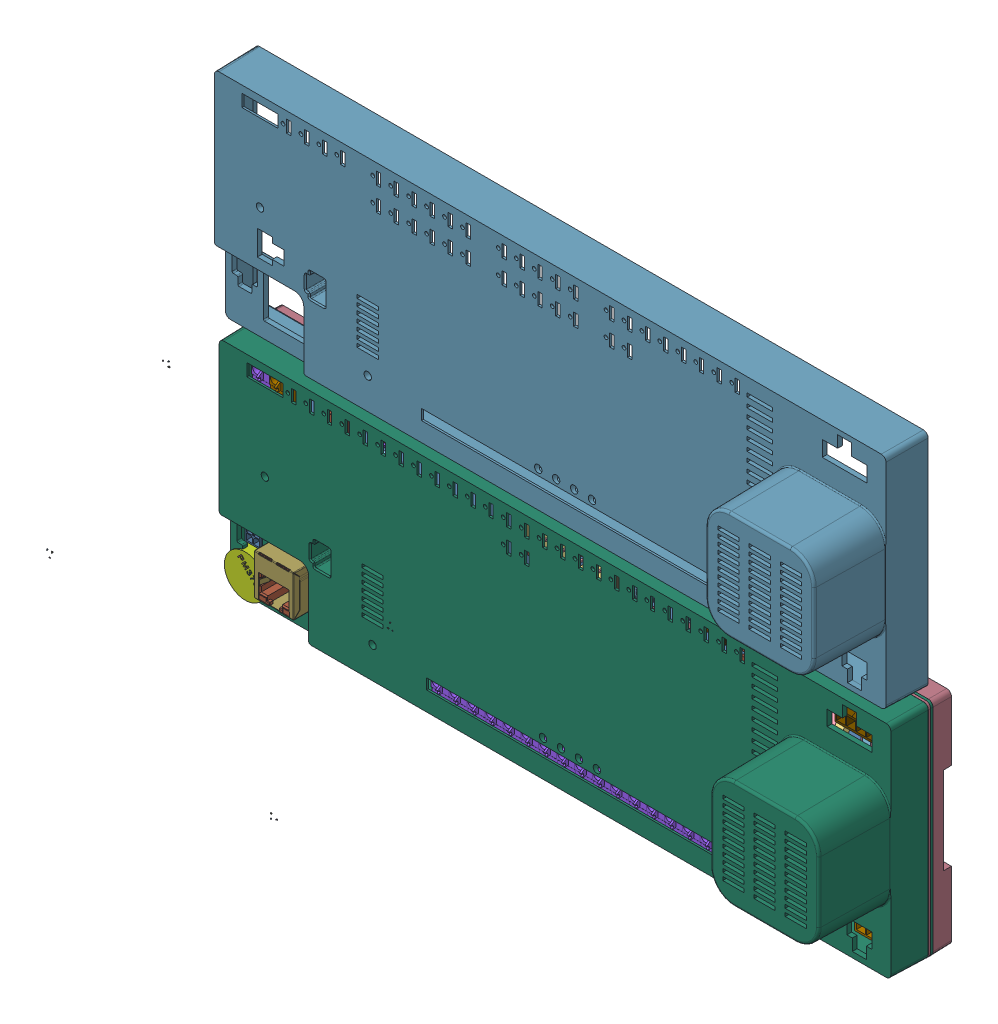
SolidWorks assembly _SC944D, configuration Default. Lengths in mm. (continued)
Components (placement in the parent): (continued)
- U10-1: U10 [Default] at origin size (22 22 1.6) (continued)
  - User_Library-LQFP144-1: User_Library-LQFP144 [Default] at (60.232 23.8429 0) x (-1 0 0) z (0 1 0) size (22 1.6 22) (continued)
    - User_Library-LQFP144_Assu_Fuss_LQFP144-1: User_Library-LQFP144_Assu_Fuss_LQFP144 [Default] at (10 0 0) size (1 0.89 17.72) (continued)
      - User_Library-LQFP144_Fuss_LQFP144-291: User_Library-LQFP144_Fuss_LQFP144 [Default] at (0 0 -7.75) size (1 0.89 0.22)
      - User_Library-LQFP144_Fuss_LQFP144-292: User_Library-LQFP144_Fuss_LQFP144 [Default] at (0 0 1.25) size (1 0.89 0.22)
      - User_Library-LQFP144_Fuss_LQFP144-293: User_Library-LQFP144_Fuss_LQFP144 [Default] at (0 0 5.25) size (1 0.89 0.22)
      - User_Library-LQFP144_Fuss_LQFP144-294: User_Library-LQFP144_Fuss_LQFP144 [Default] at (0 0 -0.75) size (1 0.89 0.22)
      - User_Library-LQFP144_Fuss_LQFP144-295: User_Library-LQFP144_Fuss_LQFP144 [Default] at (0 0 5.75) size (1 0.89 0.22)
      - User_Library-LQFP144_Fuss_LQFP144-296: User_Library-LQFP144_Fuss_LQFP144 [Default] at (0 0 2.75) size (1 0.89 0.22)
      - User_Library-LQFP144_Fuss_LQFP144-297: User_Library-LQFP144_Fuss_LQFP144 [Default] at (0 0 -1.75) size (1 0.89 0.22)
      - User_Library-LQFP144_Fuss_LQFP144-298: User_Library-LQFP144_Fuss_LQFP144 [Default] at (0 0 2.25) size (1 0.89 0.22)
      - User_Library-LQFP144_Fuss_LQFP144-299: User_Library-LQFP144_Fuss_LQFP144 [Default] at (0 0 1.25) size (1 0.89 0.22)
      - User_Library-LQFP144_Fuss_LQFP144-300: User_Library-LQFP144_Fuss_LQFP144 [Default] at (0 0 3.75) size (1 0.89 0.22)
      - User_Library-LQFP144_Fuss_LQFP144-301: User_Library-LQFP144_Fuss_LQFP144 [Default] at (0 0 -3.75) size (1 0.89 0.22)
      - User_Library-LQFP144_Fuss_LQFP144-302: User_Library-LQFP144_Fuss_LQFP144 [Default] at (0 0 0.75) size (1 0.89 0.22)
      - User_Library-LQFP144_Fuss_LQFP144-303: User_Library-LQFP144_Fuss_LQFP144 [Default] at (0 0 -6.75) size (1 0.89 0.22)
      - User_Library-LQFP144_Fuss_LQFP144-304: User_Library-LQFP144_Fuss_LQFP144 [Default] at (0 0 -3.25) size (1 0.89 0.22)
      - User_Library-LQFP144_Fuss_LQFP144-305: User_Library-LQFP144_Fuss_LQFP144 [Default] at (0 0 2.25) size (1 0.89 0.22)
      - User_Library-LQFP144_Fuss_LQFP144-306: User_Library-LQFP144_Fuss_LQFP144 [Default] at (0 0 -5.75) size (1 0.89 0.22)
      - User_Library-LQFP144_Fuss_LQFP144-307: User_Library-LQFP144_Fuss_LQFP144 [Default] at (0 0 0.25) size (1 0.89 0.22)
      - User_Library-LQFP144_Fuss_LQFP144-308: User_Library-LQFP144_Fuss_LQFP144 [Default] at (0 0 1.75) size (1 0.89 0.22)
      - User_Library-LQFP144_Fuss_LQFP144-309: User_Library-LQFP144_Fuss_LQFP144 [Default] at (0 0 -5.75) size (1 0.89 0.22)
      - User_Library-LQFP144_Fuss_LQFP144-310: User_Library-LQFP144_Fuss_LQFP144 [Default] at (0 0 -3.25) size (1 0.89 0.22)
      - User_Library-LQFP144_Fuss_LQFP144-311: User_Library-LQFP144_Fuss_LQFP144 [Default] at (0 0 -0.75) size (1 0.89 0.22)
      - User_Library-LQFP144_Fuss_LQFP144-312: User_Library-LQFP144_Fuss_LQFP144 [Default] at (0 0 -1.75) size (1 0.89 0.22)
      - User_Library-LQFP144_Fuss_LQFP144-313: User_Library-LQFP144_Fuss_LQFP144 [Default] at (0 0 2.25) size (1 0.89 0.22)
      - User_Library-LQFP144_Fuss_LQFP144-314: User_Library-LQFP144_Fuss_LQFP144 [Default] at (0 0 1.25) size (1 0.89 0.22)
      - User_Library-LQFP144_Fuss_LQFP144-315: User_Library-LQFP144_Fuss_LQFP144 [Default] at (0 0 4.75) size (1 0.89 0.22)
      - User_Library-LQFP144_Fuss_LQFP144-316: User_Library-LQFP144_Fuss_LQFP144 [Default] at (0 0 4.25) size (1 0.89 0.22)
      - User_Library-LQFP144_Fuss_LQFP144-317: User_Library-LQFP144_Fuss_LQFP144 [Default] at (0 0 -2.25) size (1 0.89 0.22)
      - User_Library-LQFP144_Fuss_LQFP144-318: User_Library-LQFP144_Fuss_LQFP144 [Default] at (0 0 3.75) size (1 0.89 0.22)
      - User_Library-LQFP144_Fuss_LQFP144-319: User_Library-LQFP144_Fuss_LQFP144 [Default] at (0 0 4.25) size (1 0.89 0.22)
      - User_Library-LQFP144_Fuss_LQFP144-320: User_Library-LQFP144_Fuss_LQFP144 [Default] at (0 0 -1.25) size (1 0.89 0.22)
      - User_Library-LQFP144_Fuss_LQFP144-321: User_Library-LQFP144_Fuss_LQFP144 [Default] at (0 0 -3.75) size (1 0.89 0.22)
      - User_Library-LQFP144_Fuss_LQFP144-322: User_Library-LQFP144_Fuss_LQFP144 [Default] at (0 0 -2.25) size (1 0.89 0.22)
      - User_Library-LQFP144_Fuss_LQFP144-323: User_Library-LQFP144_Fuss_LQFP144 [Default] at (0 0 3.25) size (1 0.89 0.22)
      - User_Library-LQFP144_Fuss_LQFP144-324: User_Library-LQFP144_Fuss_LQFP144 [Default] at (0 0 1.25) size (1 0.89 0.22)
      - User_Library-LQFP144_Fuss_LQFP144-325: User_Library-LQFP144_Fuss_LQFP144 [Default] at (0 0 0.25) size (1 0.89 0.22)
      - User_Library-LQFP144_Fuss_LQFP144-326: User_Library-LQFP144_Fuss_LQFP144 [Default] at (0 0 2.75) size (1 0.89 0.22)
      - User_Library-LQFP144_Fuss_LQFP144-327: User_Library-LQFP144_Fuss_LQFP144 [Default] at (0 0 -2.75) size (1 0.89 0.22)
      - User_Library-LQFP144_Fuss_LQFP144-328: User_Library-LQFP144_Fuss_LQFP144 [Default] at (0 0 -3.75) size (1 0.89 0.22)
      - User_Library-LQFP144_Fuss_LQFP144-329: User_Library-LQFP144_Fuss_LQFP144 [Default] at (0 0 -0.25) size (1 0.89 0.22)
      - User_Library-LQFP144_Fuss_LQFP144-330: User_Library-LQFP144_Fuss_LQFP144 [Default] at (0 0 -2.75) size (1 0.89 0.22)
      - User_Library-LQFP144_Fuss_LQFP144-331: User_Library-LQFP144_Fuss_LQFP144 [Default] at (0 0 -5.25) size (1 0.89 0.22)
      - User_Library-LQFP144_Fuss_LQFP144-332: User_Library-LQFP144_Fuss_LQFP144 [Default] at (0 0 -2.25) size (1 0.89 0.22)
      - User_Library-LQFP144_Fuss_LQFP144-333: User_Library-LQFP144_Fuss_LQFP144 [Default] at (0 0 0.75) size (1 0.89 0.22)
      - User_Library-LQFP144_Fuss_LQFP144-334: User_Library-LQFP144_Fuss_LQFP144 [Default] at (0 0 5.25) size (1 0.89 0.22)
      - User_Library-LQFP144_Fuss_LQFP144-335: User_Library-LQFP144_Fuss_LQFP144 [Default] at (0 0 -1.25) size (1 0.89 0.22)
      - User_Library-LQFP144_Fuss_LQFP144-336: User_Library-LQFP144_Fuss_LQFP144 [Default] at (0 0 2.25) size (1 0.89 0.22)
      - User_Library-LQFP144_Fuss_LQFP144-337: User_Library-LQFP144_Fuss_LQFP144 [Default] at (0 0 3.75) size (1 0.89 0.22)
      - User_Library-LQFP144_Fuss_LQFP144-338: User_Library-LQFP144_Fuss_LQFP144 [Default] at (0 0 2.25) size (1 0.89 0.22)
      - User_Library-LQFP144_Fuss_LQFP144-339: User_Library-LQFP144_Fuss_LQFP144 [Default] at (0 0 4.75) size (1 0.89 0.22)
      - User_Library-LQFP144_Fuss_LQFP144-340: User_Library-LQFP144_Fuss_LQFP144 [Default] at (0 0 0.75) size (1 0.89 0.22)
      - User_Library-LQFP144_Fuss_LQFP144-341: User_Library-LQFP144_Fuss_LQFP144 [Default] at (0 0 3.25) size (1 0.89 0.22)
      - User_Library-LQFP144_Fuss_LQFP144-342: User_Library-LQFP144_Fuss_LQFP144 [Default] at (0 0 2.75) size (1 0.89 0.22)
    - User_Library-LQFP144_Assu_Fuss_LQFP144-2: User_Library-LQFP144_Assu_Fuss_LQFP144 [Default] at (0 0 -10) x (0 0 -1) z (1 0 0) size (1 0.89 17.72)
      - User_Library-LQFP144_Fuss_LQFP144-1: User_Library-LQFP144_Fuss_LQFP144 [Default] at (0 0 3.25) size (1 0.89 0.22)
      - User_Library-LQFP144_Fuss_LQFP144-2: User_Library-LQFP144_Fuss_LQFP144 [Default] at (0 0 -5.75) size (1 0.89 0.22)
      - User_Library-LQFP144_Fuss_LQFP144-3: User_Library-LQFP144_Fuss_LQFP144 [Default] at (0 0 -3.75) size (1 0.89 0.22)
      - User_Library-LQFP144_Fuss_LQFP144-4: User_Library-LQFP144_Fuss_LQFP144 [Default] at (0 0 -0.25) size (1 0.89 0.22)
      - User_Library-LQFP144_Fuss_LQFP144-5: User_Library-LQFP144_Fuss_LQFP144 [Default] at (0 0 -5.25) size (1 0.89 0.22)
      - User_Library-LQFP144_Fuss_LQFP144-6: User_Library-LQFP144_Fuss_LQFP144 [Default] at (0 0 -8.25) size (1 0.89 0.22)
      - User_Library-LQFP144_Fuss_LQFP144-7: User_Library-LQFP144_Fuss_LQFP144 [Default] at (0 0 -0.25) size (1 0.89 0.22)
      - User_Library-LQFP144_Fuss_LQFP144-8: User_Library-LQFP144_Fuss_LQFP144 [Default] at (0 0 -3.75) size (1 0.89 0.22)
      - User_Library-LQFP144_Fuss_LQFP144-9: User_Library-LQFP144_Fuss_LQFP144 [Default] at (0 0 -0.25) size (1 0.89 0.22)
      - User_Library-LQFP144_Fuss_LQFP144-10: User_Library-LQFP144_Fuss_LQFP144 [Default] at (0 0 6.75) size (1 0.89 0.22)
      - User_Library-LQFP144_Fuss_LQFP144-11: User_Library-LQFP144_Fuss_LQFP144 [Default] at (0 0 -3.75) size (1 0.89 0.22)
      - User_Library-LQFP144_Fuss_LQFP144-12: User_Library-LQFP144_Fuss_LQFP144 [Default] at (0 0 4.25) size (1 0.89 0.22)
      - User_Library-LQFP144_Fuss_LQFP144-13: User_Library-LQFP144_Fuss_LQFP144 [Default] at (0 0 0.75) size (1 0.89 0.22)
      - User_Library-LQFP144_Fuss_LQFP144-14: User_Library-LQFP144_Fuss_LQFP144 [Default] at (0 0 7.75) size (1 0.89 0.22)
      - User_Library-LQFP144_Fuss_LQFP144-15: User_Library-LQFP144_Fuss_LQFP144 [Default] at (0 0 1.75) size (1 0.89 0.22)
      - User_Library-LQFP144_Fuss_LQFP144-16: User_Library-LQFP144_Fuss_LQFP144 [Default] at (0 0 -2.25) size (1 0.89 0.22)
      - User_Library-LQFP144_Fuss_LQFP144-17: User_Library-LQFP144_Fuss_LQFP144 [Default] at (0 0 -2.75) size (1 0.89 0.22)
      - User_Library-LQFP144_Fuss_LQFP144-18: User_Library-LQFP144_Fuss_LQFP144 [Default] at (0 0 -4.25) size (1 0.89 0.22)
      - User_Library-LQFP144_Fuss_LQFP144-19: User_Library-LQFP144_Fuss_LQFP144 [Default] at (0 0 3.25) size (1 0.89 0.22)
      - User_Library-LQFP144_Fuss_LQFP144-20: User_Library-LQFP144_Fuss_LQFP144 [Default] at (0 0 -1.75) size (1 0.89 0.22)
      - User_Library-LQFP144_Fuss_LQFP144-21: User_Library-LQFP144_Fuss_LQFP144 [Default] at (0 0 -1.75) size (1 0.89 0.22)
      - User_Library-LQFP144_Fuss_LQFP144-22: User_Library-LQFP144_Fuss_LQFP144 [Default] at (0 0 2.75) size (1 0.89 0.22)
      - User_Library-LQFP144_Fuss_LQFP144-23: User_Library-LQFP144_Fuss_LQFP144 [Default] at (0 0 -2.75) size (1 0.89 0.22)
      - User_Library-LQFP144_Fuss_LQFP144-24: User_Library-LQFP144_Fuss_LQFP144 [Default] at (0 0 -3.75) size (1 0.89 0.22)
      - User_Library-LQFP144_Fuss_LQFP144-25: User_Library-LQFP144_Fuss_LQFP144 [Default] at (0 0 -5.75) size (1 0.89 0.22)
      - User_Library-LQFP144_Fuss_LQFP144-26: User_Library-LQFP144_Fuss_LQFP144 [Default] at (0 0 0.75) size (1 0.89 0.22)
      - User_Library-LQFP144_Fuss_LQFP144-27: User_Library-LQFP144_Fuss_LQFP144 [Default] at (0 0 -6.25) size (1 0.89 0.22)
      - User_Library-LQFP144_Fuss_LQFP144-28: User_Library-LQFP144_Fuss_LQFP144 [Default] at (0 0 -2.75) size (1 0.89 0.22)
      - User_Library-LQFP144_Fuss_LQFP144-29: User_Library-LQFP144_Fuss_LQFP144 [Default] at (0 0 1.25) size (1 0.89 0.22)
      - User_Library-LQFP144_Fuss_LQFP144-30: User_Library-LQFP144_Fuss_LQFP144 [Default] at (0 0 -0.25) size (1 0.89 0.22)
      - User_Library-LQFP144_Fuss_LQFP144-31: User_Library-LQFP144_Fuss_LQFP144 [Default] at (0 0 -1.25) size (1 0.89 0.22)
      - User_Library-LQFP144_Fuss_LQFP144-32: User_Library-LQFP144_Fuss_LQFP144 [Default] at (0 0 5.25) size (1 0.89 0.22)
      - User_Library-LQFP144_Fuss_LQFP144-33: User_Library-LQFP144_Fuss_LQFP144 [Default] at (0 0 8.25) size (1 0.89 0.22)
      - User_Library-LQFP144_Fuss_LQFP144-34: User_Library-LQFP144_Fuss_LQFP144 [Default] at (0 0 -6.25) size (1 0.89 0.22)
      - User_Library-LQFP144_Fuss_LQFP144-35: User_Library-LQFP144_Fuss_LQFP144 [Default] at (0 0 -0.75) size (1 0.89 0.22)
      - User_Library-LQFP144_Fuss_LQFP144-36: User_Library-LQFP144_Fuss_LQFP144 [Default] at (0 0 -8.75) size (1 0.89 0.22)
      - User_Library-LQFP144_Fuss_LQFP144-37: User_Library-LQFP144_Fuss_LQFP144 [Default] at (0 0 -1.25) size (1 0.89 0.22)
      - User_Library-LQFP144_Fuss_LQFP144-38: User_Library-LQFP144_Fuss_LQFP144 [Default] at (0 0 -1.25) size (1 0.89 0.22)
      - User_Library-LQFP144_Fuss_LQFP144-39: User_Library-LQFP144_Fuss_LQFP144 [Default] at (0 0 -2.75) size (1 0.89 0.22)
      - User_Library-LQFP144_Fuss_LQFP144-40: User_Library-LQFP144_Fuss_LQFP144 [Default] at (0 0 -2.75) size (1 0.89 0.22)
      - User_Library-LQFP144_Fuss_LQFP144-41: User_Library-LQFP144_Fuss_LQFP144 [Default] at (0 0 2.25) size (1 0.89 0.22)
      - User_Library-LQFP144_Fuss_LQFP144-42: User_Library-LQFP144_Fuss_LQFP144 [Default] at (0 0 3.75) size (1 0.89 0.22)
      - User_Library-LQFP144_Fuss_LQFP144-43: User_Library-LQFP144_Fuss_LQFP144 [Default] at (0 0 0.75) size (1 0.89 0.22)
      - User_Library-LQFP144_Fuss_LQFP144-44: User_Library-LQFP144_Fuss_LQFP144 [Default] at (0 0 0.75) size (1 0.89 0.22)
      - User_Library-LQFP144_Fuss_LQFP144-45: User_Library-LQFP144_Fuss_LQFP144 [Default] at (0 0 1.25) size (1 0.89 0.22)
      - User_Library-LQFP144_Fuss_LQFP144-46: User_Library-LQFP144_Fuss_LQFP144 [Default] at (0 0 1.75) size (1 0.89 0.22)
      - User_Library-LQFP144_Fuss_LQFP144-47: User_Library-LQFP144_Fuss_LQFP144 [Default] at (0 0 3.25) size (1 0.89 0.22)
      - User_Library-LQFP144_Fuss_LQFP144-48: User_Library-LQFP144_Fuss_LQFP144 [Default] at (0 0 -3.25) size (1 0.89 0.22)
      - User_Library-LQFP144_Fuss_LQFP144-49: User_Library-LQFP144_Fuss_LQFP144 [Default] at (0 0 5.75) size (1 0.89 0.22)
      - User_Library-LQFP144_Fuss_LQFP144-50: User_Library-LQFP144_Fuss_LQFP144 [Default] at (0 0 4.25) size (1 0.89 0.22)
      - User_Library-LQFP144_Fuss_LQFP144-51: User_Library-LQFP144_Fuss_LQFP144 [Default] at (0 0 3.25) size (1 0.89 0.22)
      - User_Library-LQFP144_Fuss_LQFP144-52: User_Library-LQFP144_Fuss_LQFP144 [Default] at (0 0 6.25) size (1 0.89 0.22)
      - User_Library-LQFP144_Fuss_LQFP144-53: User_Library-LQFP144_Fuss_LQFP144 [Default] at (0 0 -5.25) size (1 0.89 0.22)
      - User_Library-LQFP144_Fuss_LQFP144-54: User_Library-LQFP144_Fuss_LQFP144 [Default] at (0 0 -6.75) size (1 0.89 0.22)
      - User_Library-LQFP144_Fuss_LQFP144-55: User_Library-LQFP144_Fuss_LQFP144 [Default] at (0 0 -0.75) size (1 0.89 0.22)
      - User_Library-LQFP144_Fuss_LQFP144-56: User_Library-LQFP144_Fuss_LQFP144 [Default] at (0 0 1.75) size (1 0.89 0.22)
      - User_Library-LQFP144_Fuss_LQFP144-57: User_Library-LQFP144_Fuss_LQFP144 [Default] at (0 0 -3.25) size (1 0.89 0.22)
      - User_Library-LQFP144_Fuss_LQFP144-58: User_Library-LQFP144_Fuss_LQFP144 [Default] at (0 0 -4.25) size (1 0.89 0.22)
      - User_Library-LQFP144_Fuss_LQFP144-59: User_Library-LQFP144_Fuss_LQFP144 [Default] at (0 0 -5.25) size (1 0.89 0.22)
      - User_Library-LQFP144_Fuss_LQFP144-60: User_Library-LQFP144_Fuss_LQFP144 [Default] at (0 0 -1.25) size (1 0.89 0.22)
      - User_Library-LQFP144_Fuss_LQFP144-61: User_Library-LQFP144_Fuss_LQFP144 [Default] at (0 0 -0.75) size (1 0.89 0.22)
      - User_Library-LQFP144_Fuss_LQFP144-62: User_Library-LQFP144_Fuss_LQFP144 [Default] at (0 0 -6.25) size (1 0.89 0.22)
      - User_Library-LQFP144_Fuss_LQFP144-63: User_Library-LQFP144_Fuss_LQFP144 [Default] at (0 0 4.75) size (1 0.89 0.22)
      - User_Library-LQFP144_Fuss_LQFP144-64: User_Library-LQFP144_Fuss_LQFP144 [Default] at (0 0 3.25) size (1 0.89 0.22)
      - User_Library-LQFP144_Fuss_LQFP144-65: User_Library-LQFP144_Fuss_LQFP144 [Default] at (0 0 4.25) size (1 0.89 0.22)
      - User_Library-LQFP144_Fuss_LQFP144-66: User_Library-LQFP144_Fuss_LQFP144 [Default] at (0 0 0.25) size (1 0.89 0.22)
      - User_Library-LQFP144_Fuss_LQFP144-67: User_Library-LQFP144_Fuss_LQFP144 [Default] at (0 0 4.25) size (1 0.89 0.22)
      - User_Library-LQFP144_Fuss_LQFP144-68: User_Library-LQFP144_Fuss_LQFP144 [Default] at (0 0 6.75) size (1 0.89 0.22)
      - User_Library-LQFP144_Fuss_LQFP144-69: User_Library-LQFP144_Fuss_LQFP144 [Default] at (0 0 0.25) size (1 0.89 0.22)
      - User_Library-LQFP144_Fuss_LQFP144-70: User_Library-LQFP144_Fuss_LQFP144 [Default] at (0 0 0.25) size (1 0.89 0.22)
      - User_Library-LQFP144_Fuss_LQFP144-71: User_Library-LQFP144_Fuss_LQFP144 [Default] at (0 0 -1.25) size (1 0.89 0.22)
      - User_Library-LQFP144_Fuss_LQFP144-72: User_Library-LQFP144_Fuss_LQFP144 [Default] at (0 0 -3.75) size (1 0.89 0.22)
      - User_Library-LQFP144_Fuss_LQFP144-73: User_Library-LQFP144_Fuss_LQFP144 [Default] at (0 0 -0.25) size (1 0.89 0.22)
      - User_Library-LQFP144_Fuss_LQFP144-74: User_Library-LQFP144_Fuss_LQFP144 [Default] at (0 0 1.25) size (1 0.89 0.22)
      - User_Library-LQFP144_Fuss_LQFP144-75: User_Library-LQFP144_Fuss_LQFP144 [Default] at (0 0 0.75) size (1 0.89 0.22)
      - User_Library-LQFP144_Fuss_LQFP144-76: User_Library-LQFP144_Fuss_LQFP144 [Default] at (0 0 -7.75) size (1 0.89 0.22)
      - User_Library-LQFP144_Fuss_LQFP144-77: User_Library-LQFP144_Fuss_LQFP144 [Default] at (0 0 -3.25) size (1 0.89 0.22)
      - User_Library-LQFP144_Fuss_LQFP144-78: User_Library-LQFP144_Fuss_LQFP144 [Default] at (0 0 2.75) size (1 0.89 0.22)
      - User_Library-LQFP144_Fuss_LQFP144-79: User_Library-LQFP144_Fuss_LQFP144 [Default] at (0 0 4.75) size (1 0.89 0.22)
      - User_Library-LQFP144_Fuss_LQFP144-80: User_Library-LQFP144_Fuss_LQFP144 [Default] at (0 0 -7.25) size (1 0.89 0.22)
      - User_Library-LQFP144_Fuss_LQFP144-81: User_Library-LQFP144_Fuss_LQFP144 [Default] at (0 0 0.75) size (1 0.89 0.22)
      - User_Library-LQFP144_Fuss_LQFP144-82: User_Library-LQFP144_Fuss_LQFP144 [Default] at (0 0 0.75) size (1 0.89 0.22)
      - User_Library-LQFP144_Fuss_LQFP144-83: User_Library-LQFP144_Fuss_LQFP144 [Default] at (0 0 -0.75) size (1 0.89 0.22)
      - User_Library-LQFP144_Fuss_LQFP144-84: User_Library-LQFP144_Fuss_LQFP144 [Default] at (0 0 6.75) size (1 0.89 0.22)
      - User_Library-LQFP144_Fuss_LQFP144-85: User_Library-LQFP144_Fuss_LQFP144 [Default] at (0 0 -3.25) size (1 0.89 0.22)
      - User_Library-LQFP144_Fuss_LQFP144-86: User_Library-LQFP144_Fuss_LQFP144 [Default] at (0 0 3.75) size (1 0.89 0.22)
      - User_Library-LQFP144_Fuss_LQFP144-87: User_Library-LQFP144_Fuss_LQFP144 [Default] at (0 0 -0.75) size (1 0.89 0.22)
      - User_Library-LQFP144_Fuss_LQFP144-88: User_Library-LQFP144_Fuss_LQFP144 [Default] at (0 0 -1.75) size (1 0.89 0.22)
      - User_Library-LQFP144_Fuss_LQFP144-89: User_Library-LQFP144_Fuss_LQFP144 [Default] at (0 0 7.25) size (1 0.89 0.22)
      - User_Library-LQFP144_Fuss_LQFP144-90: User_Library-LQFP144_Fuss_LQFP144 [Default] at (0 0 0.75) size (1 0.89 0.22)
      - User_Library-LQFP144_Fuss_LQFP144-91: User_Library-LQFP144_Fuss_LQFP144 [Default] at (0 0 0.25) size (1 0.89 0.22)
      - User_Library-LQFP144_Fuss_LQFP144-92: User_Library-LQFP144_Fuss_LQFP144 [Default] at (0 0 0.25) size (1 0.89 0.22)
      - User_Library-LQFP144_Fuss_LQFP144-93: User_Library-LQFP144_Fuss_LQFP144 [Default] at (0 0 0.25) size (1 0.89 0.22)
      - User_Library-LQFP144_Fuss_LQFP144-94: User_Library-LQFP144_Fuss_LQFP144 [Default] at (0 0 1.75) size (1 0.89 0.22)
      - User_Library-LQFP144_Fuss_LQFP144-95: User_Library-LQFP144_Fuss_LQFP144 [Default] at (0 0 3.25) size (1 0.89 0.22)
      - User_Library-LQFP144_Fuss_LQFP144-96: User_Library-LQFP144_Fuss_LQFP144 [Default] at (0 0 -2.75) size (1 0.89 0.22)
      - User_Library-LQFP144_Fuss_LQFP144-97: User_Library-LQFP144_Fuss_LQFP144 [Default] at (0 0 -1.75) size (1 0.89 0.22)
      - User_Library-LQFP144_Fuss_LQFP144-98: User_Library-LQFP144_Fuss_LQFP144 [Default] at (0 0 4.75) size (1 0.89 0.22)
      - User_Library-LQFP144_Fuss_LQFP144-99: User_Library-LQFP144_Fuss_LQFP144 [Default] at (0 0 1.25) size (1 0.89 0.22)
      - User_Library-LQFP144_Fuss_LQFP144-100: User_Library-LQFP144_Fuss_LQFP144 [Default] at (0 0 4.75) size (1 0.89 0.22)
      - User_Library-LQFP144_Fuss_LQFP144-101: User_Library-LQFP144_Fuss_LQFP144 [Default] at (0 0 2.25) size (1 0.89 0.22)
      - User_Library-LQFP144_Fuss_LQFP144-102: User_Library-LQFP144_Fuss_LQFP144 [Default] at (0 0 2.25) size (1 0.89 0.22)
      - User_Library-LQFP144_Fuss_LQFP144-103: User_Library-LQFP144_Fuss_LQFP144 [Default] at (0 0 -2.75) size (1 0.89 0.22)
      - User_Library-LQFP144_Fuss_LQFP144-104: User_Library-LQFP144_Fuss_LQFP144 [Default] at (0 0 1.75) size (1 0.89 0.22)
      - User_Library-LQFP144_Fuss_LQFP144-105: User_Library-LQFP144_Fuss_LQFP144 [Default] at (0 0 7.25) size (1 0.89 0.22)
      - User_Library-LQFP144_Fuss_LQFP144-106: User_Library-LQFP144_Fuss_LQFP144 [Default] at (0 0 4.25) size (1 0.89 0.22)
      - User_Library-LQFP144_Fuss_LQFP144-107: User_Library-LQFP144_Fuss_LQFP144 [Default] at (0 0 7.75) size (1 0.89 0.22)
      - User_Library-LQFP144_Fuss_LQFP144-108: User_Library-LQFP144_Fuss_LQFP144 [Default] at (0 0 4.25) size (1 0.89 0.22)
      - User_Library-LQFP144_Fuss_LQFP144-109: User_Library-LQFP144_Fuss_LQFP144 [Default] at (0 0 7.25) size (1 0.89 0.22)
      - User_Library-LQFP144_Fuss_LQFP144-110: User_Library-LQFP144_Fuss_LQFP144 [Default] at (0 0 1.25) size (1 0.89 0.22)
      - User_Library-LQFP144_Fuss_LQFP144-111: User_Library-LQFP144_Fuss_LQFP144 [Default] at (0 0 7.25) size (1 0.89 0.22)
      - User_Library-LQFP144_Fuss_LQFP144-112: User_Library-LQFP144_Fuss_LQFP144 [Default] at (0 0 5.25) size (1 0.89 0.22)
      - User_Library-LQFP144_Fuss_LQFP144-113: User_Library-LQFP144_Fuss_LQFP144 [Default] at (0 0 6.75) size (1 0.89 0.22)
      - User_Library-LQFP144_Fuss_LQFP144-114: User_Library-LQFP144_Fuss_LQFP144 [Default] at (0 0 -6.25) size (1 0.89 0.22)
      - User_Library-LQFP144_Fuss_LQFP144-115: User_Library-LQFP144_Fuss_LQFP144 [Default] at (0 0 -0.25) size (1 0.89 0.22)
      - User_Library-LQFP144_Fuss_LQFP144-116: User_Library-LQFP144_Fuss_LQFP144 [Default] at (0 0 0.25) size (1 0.89 0.22)
      - User_Library-LQFP144_Fuss_LQFP144-117: User_Library-LQFP144_Fuss_LQFP144 [Default] at (0 0 8.25) size (1 0.89 0.22)
      - User_Library-LQFP144_Fuss_LQFP144-118: User_Library-LQFP144_Fuss_LQFP144 [Default] at (0 0 -4.75) size (1 0.89 0.22)
      - User_Library-LQFP144_Fuss_LQFP144-119: User_Library-LQFP144_Fuss_LQFP144 [Default] at (0 0 -2.25) size (1 0.89 0.22)
      - User_Library-LQFP144_Fuss_LQFP144-120: User_Library-LQFP144_Fuss_LQFP144 [Default] at (0 0 -6.75) size (1 0.89 0.22)
      - User_Library-LQFP144_Fuss_LQFP144-121: User_Library-LQFP144_Fuss_LQFP144 [Default] at (0 0 -1.75) size (1 0.89 0.22)
      - User_Library-LQFP144_Fuss_LQFP144-122: User_Library-LQFP144_Fuss_LQFP144 [Default] at (0 0 -7.25) size (1 0.89 0.22)
      - User_Library-LQFP144_Fuss_LQFP144-123: User_Library-LQFP144_Fuss_LQFP144 [Default] at (0 0 -5.25) size (1 0.89 0.22)
      - User_Library-LQFP144_Fuss_LQFP144-124: User_Library-LQFP144_Fuss_LQFP144 [Default] at (0 0 -5.75) size (1 0.89 0.22)
      - User_Library-LQFP144_Fuss_LQFP144-125: User_Library-LQFP144_Fuss_LQFP144 [Default] at (0 0 2.75) size (1 0.89 0.22)
      - User_Library-LQFP144_Fuss_LQFP144-126: User_Library-LQFP144_Fuss_LQFP144 [Default] at (0 0 1.75) size (1 0.89 0.22)
      - User_Library-LQFP144_Fuss_LQFP144-127: User_Library-LQFP144_Fuss_LQFP144 [Default] at (0 0 0.25) size (1 0.89 0.22)
      - User_Library-LQFP144_Fuss_LQFP144-128: User_Library-LQFP144_Fuss_LQFP144 [Default] at (0 0 -3.25) size (1 0.89 0.22)
      - User_Library-LQFP144_Fuss_LQFP144-129: User_Library-LQFP144_Fuss_LQFP144 [Default] at (0 0 3.25) size (1 0.89 0.22)
      - User_Library-LQFP144_Fuss_LQFP144-130: User_Library-LQFP144_Fuss_LQFP144 [Default] at (0 0 -2.75) size (1 0.89 0.22)
      - User_Library-LQFP144_Fuss_LQFP144-131: User_Library-LQFP144_Fuss_LQFP144 [Default] at (0 0 3.75) size (1 0.89 0.22)
      - User_Library-LQFP144_Fuss_LQFP144-132: User_Library-LQFP144_Fuss_LQFP144 [Default] at (0 0 0.25) size (1 0.89 0.22)
      - User_Library-LQFP144_Fuss_LQFP144-133: User_Library-LQFP144_Fuss_LQFP144 [Default] at (0 0 2.25) size (1 0.89 0.22)
      - User_Library-LQFP144_Fuss_LQFP144-134: User_Library-LQFP144_Fuss_LQFP144 [Default] at (0 0 -1.25) size (1 0.89 0.22)
      - User_Library-LQFP144_Fuss_LQFP144-135: User_Library-LQFP144_Fuss_LQFP144 [Default] at (0 0 -0.75) size (1 0.89 0.22)
      - User_Library-LQFP144_Fuss_LQFP144-136: User_Library-LQFP144_Fuss_LQFP144 [Default] at (0 0 -4.25) size (1 0.89 0.22)
      - User_Library-LQFP144_Fuss_LQFP144-137: User_Library-LQFP144_Fuss_LQFP144 [Default] at (0 0 1.75) size (1 0.89 0.22)
      - User_Library-LQFP144_Fuss_LQFP144-138: User_Library-LQFP144_Fuss_LQFP144 [Default] at (0 0 -1.25) size (1 0.89 0.22)
      - User_Library-LQFP144_Fuss_LQFP144-139: User_Library-LQFP144_Fuss_LQFP144 [Default] at (0 0 -1.75) size (1 0.89 0.22)
      - User_Library-LQFP144_Fuss_LQFP144-140: User_Library-LQFP144_Fuss_LQFP144 [Default] at (0 0 4.25) size (1 0.89 0.22)
      - User_Library-LQFP144_Fuss_LQFP144-141: User_Library-LQFP144_Fuss_LQFP144 [Default] at (0 0 -2.25) size (1 0.89 0.22)
      - User_Library-LQFP144_Fuss_LQFP144-142: User_Library-LQFP144_Fuss_LQFP144 [Default] at (0 0 5.25) size (1 0.89 0.22)
      - User_Library-LQFP144_Fuss_LQFP144-143: User_Library-LQFP144_Fuss_LQFP144 [Default] at (0 0 2.75) size (1 0.89 0.22)
      - User_Library-LQFP144_Fuss_LQFP144-144: User_Library-LQFP144_Fuss_LQFP144 [Default] at (0 0 -1.75) size (1 0.89 0.22)
      - User_Library-LQFP144_Fuss_LQFP144-145: User_Library-LQFP144_Fuss_LQFP144 [Default] at (0 0 -0.25) size (1 0.89 0.22)
      - User_Library-LQFP144_Fuss_LQFP144-146: User_Library-LQFP144_Fuss_LQFP144 [Default] at (0 0 0.75) size (1 0.89 0.22)
      - User_Library-LQFP144_Fuss_LQFP144-147: User_Library-LQFP144_Fuss_LQFP144 [Default] at (0 0 -0.25) size (1 0.89 0.22)
      - User_Library-LQFP144_Fuss_LQFP144-148: User_Library-LQFP144_Fuss_LQFP144 [Default] at (0 0 3.75) size (1 0.89 0.22)
      - User_Library-LQFP144_Fuss_LQFP144-149: User_Library-LQFP144_Fuss_LQFP144 [Default] at (0 0 2.75) size (1 0.89 0.22)
      - User_Library-LQFP144_Fuss_LQFP144-150: User_Library-LQFP144_Fuss_LQFP144 [Default] at (0 0 2.75) size (1 0.89 0.22)
      - User_Library-LQFP144_Fuss_LQFP144-151: User_Library-LQFP144_Fuss_LQFP144 [Default] at (0 0 6.25) size (1 0.89 0.22)
      - User_Library-LQFP144_Fuss_LQFP144-152: User_Library-LQFP144_Fuss_LQFP144 [Default] at (0 0 2.25) size (1 0.89 0.22)
      - User_Library-LQFP144_Fuss_LQFP144-153: User_Library-LQFP144_Fuss_LQFP144 [Default] at (0 0 -0.75) size (1 0.89 0.22)
      - User_Library-LQFP144_Fuss_LQFP144-154: User_Library-LQFP144_Fuss_LQFP144 [Default] at (0 0 -2.25) size (1 0.89 0.22)
      - User_Library-LQFP144_Fuss_LQFP144-155: User_Library-LQFP144_Fuss_LQFP144 [Default] at (0 0 -0.75) size (1 0.89 0.22)
      - User_Library-LQFP144_Fuss_LQFP144-156: User_Library-LQFP144_Fuss_LQFP144 [Default] at (0 0 -2.25) size (1 0.89 0.22)
      - User_Library-LQFP144_Fuss_LQFP144-157: User_Library-LQFP144_Fuss_LQFP144 [Default] at (0 0 -2.25) size (1 0.89 0.22)
      - User_Library-LQFP144_Fuss_LQFP144-158: User_Library-LQFP144_Fuss_LQFP144 [Default] at (0 0 0.75) size (1 0.89 0.22)
      - User_Library-LQFP144_Fuss_LQFP144-159: User_Library-LQFP144_Fuss_LQFP144 [Default] at (0 0 -4.25) size (1 0.89 0.22)
      - User_Library-LQFP144_Fuss_LQFP144-160: User_Library-LQFP144_Fuss_LQFP144 [Default] at (0 0 4.25) size (1 0.89 0.22)
      - User_Library-LQFP144_Fuss_LQFP144-161: User_Library-LQFP144_Fuss_LQFP144 [Default] at (0 0 1.25) size (1 0.89 0.22)
      - User_Library-LQFP144_Fuss_LQFP144-162: User_Library-LQFP144_Fuss_LQFP144 [Default] at (0 0 -0.25) size (1 0.89 0.22)
      - User_Library-LQFP144_Fuss_LQFP144-163: User_Library-LQFP144_Fuss_LQFP144 [Default] at (0 0 -4.25) size (1 0.89 0.22)
      - User_Library-LQFP144_Fuss_LQFP144-164: User_Library-LQFP144_Fuss_LQFP144 [Default] at (0 0 -1.25) size (1 0.89 0.22)
      - User_Library-LQFP144_Fuss_LQFP144-165: User_Library-LQFP144_Fuss_LQFP144 [Default] at (0 0 -8.25) size (1 0.89 0.22)
      - User_Library-LQFP144_Fuss_LQFP144-166: User_Library-LQFP144_Fuss_LQFP144 [Default] at (0 0 -3.25) size (1 0.89 0.22)
      - User_Library-LQFP144_Fuss_LQFP144-167: User_Library-LQFP144_Fuss_LQFP144 [Default] at (0 0 -4.75) size (1 0.89 0.22)
      - User_Library-LQFP144_Fuss_LQFP144-168: User_Library-LQFP144_Fuss_LQFP144 [Default] at (0 0 -2.25) size (1 0.89 0.22)
      - User_Library-LQFP144_Fuss_LQFP144-169: User_Library-LQFP144_Fuss_LQFP144 [Default] at (0 0 -1.25) size (1 0.89 0.22)
      - User_Library-LQFP144_Fuss_LQFP144-170: User_Library-LQFP144_Fuss_LQFP144 [Default] at (0 0 -7.25) size (1 0.89 0.22)
      - User_Library-LQFP144_Fuss_LQFP144-171: User_Library-LQFP144_Fuss_LQFP144 [Default] at (0 0 -4.25) size (1 0.89 0.22)
      - User_Library-LQFP144_Fuss_LQFP144-172: User_Library-LQFP144_Fuss_LQFP144 [Default] at (0 0 -4.25) size (1 0.89 0.22)
      - User_Library-LQFP144_Fuss_LQFP144-173: User_Library-LQFP144_Fuss_LQFP144 [Default] at (0 0 1.75) size (1 0.89 0.22)
      - User_Library-LQFP144_Fuss_LQFP144-174: User_Library-LQFP144_Fuss_LQFP144 [Default] at (0 0 0.25) size (1 0.89 0.22)
      - User_Library-LQFP144_Fuss_LQFP144-175: User_Library-LQFP144_Fuss_LQFP144 [Default] at (0 0 -0.75) size (1 0.89 0.22)
      - User_Library-LQFP144_Fuss_LQFP144-176: User_Library-LQFP144_Fuss_LQFP144 [Default] at (0 0 0.75) size (1 0.89 0.22)
      - User_Library-LQFP144_Fuss_LQFP144-177: User_Library-LQFP144_Fuss_LQFP144 [Default] at (0 0 1.75) size (1 0.89 0.22)
      - User_Library-LQFP144_Fuss_LQFP144-178: User_Library-LQFP144_Fuss_LQFP144 [Default] at (0 0 -0.75) size (1 0.89 0.22)
      - User_Library-LQFP144_Fuss_LQFP144-179: User_Library-LQFP144_Fuss_LQFP144 [Default] at (0 0 3.75) size (1 0.89 0.22)
      - User_Library-LQFP144_Fuss_LQFP144-180: User_Library-LQFP144_Fuss_LQFP144 [Default] at (0 0 4.75) size (1 0.89 0.22)
      - User_Library-LQFP144_Fuss_LQFP144-181: User_Library-LQFP144_Fuss_LQFP144 [Default] at (0 0 -0.75) size (1 0.89 0.22)
      - User_Library-LQFP144_Fuss_LQFP144-182: User_Library-LQFP144_Fuss_LQFP144 [Default] at (0 0 2.75) size (1 0.89 0.22)
      - User_Library-LQFP144_Fuss_LQFP144-183: User_Library-LQFP144_Fuss_LQFP144 [Default] at (0 0 -1.25) size (1 0.89 0.22)
      - User_Library-LQFP144_Fuss_LQFP144-184: User_Library-LQFP144_Fuss_LQFP144 [Default] at (0 0 2.75) size (1 0.89 0.22)
      - User_Library-LQFP144_Fuss_LQFP144-185: User_Library-LQFP144_Fuss_LQFP144 [Default] at (0 0 5.25) size (1 0.89 0.22)
      - User_Library-LQFP144_Fuss_LQFP144-186: User_Library-LQFP144_Fuss_LQFP144 [Default] at (0 0 -4.25) size (1 0.89 0.22)
      - User_Library-LQFP144_Fuss_LQFP144-187: User_Library-LQFP144_Fuss_LQFP144 [Default] at (0 0 -4.75) size (1 0.89 0.22)
      - User_Library-LQFP144_Fuss_LQFP144-188: User_Library-LQFP144_Fuss_LQFP144 [Default] at (0 0 -3.75) size (1 0.89 0.22)
      - User_Library-LQFP144_Fuss_LQFP144-189: User_Library-LQFP144_Fuss_LQFP144 [Default] at (0 0 -6.25) size (1 0.89 0.22)
      - User_Library-LQFP144_Fuss_LQFP144-190: User_Library-LQFP144_Fuss_LQFP144 [Default] at (0 0 0.75) size (1 0.89 0.22)
      - User_Library-LQFP144_Fuss_LQFP144-191: User_Library-LQFP144_Fuss_LQFP144 [Default] at (0 0 0.25) size (1 0.89 0.22)
      - User_Library-LQFP144_Fuss_LQFP144-192: User_Library-LQFP144_Fuss_LQFP144 [Default] at (0 0 -0.25) size (1 0.89 0.22)
      - User_Library-LQFP144_Fuss_LQFP144-193: User_Library-LQFP144_Fuss_LQFP144 [Default] at (0 0 -3.25) size (1 0.89 0.22)
      - User_Library-LQFP144_Fuss_LQFP144-194: User_Library-LQFP144_Fuss_LQFP144 [Default] at (0 0 1.75) size (1 0.89 0.22)
      - User_Library-LQFP144_Fuss_LQFP144-195: User_Library-LQFP144_Fuss_LQFP144 [Default] at (0 0 0.25) size (1 0.89 0.22)
      - User_Library-LQFP144_Fuss_LQFP144-196: User_Library-LQFP144_Fuss_LQFP144 [Default] at (0 0 5.25) size (1 0.89 0.22)
      - User_Library-LQFP144_Fuss_LQFP144-197: User_Library-LQFP144_Fuss_LQFP144 [Default] at (0 0 -1.75) size (1 0.89 0.22)
      - User_Library-LQFP144_Fuss_LQFP144-198: User_Library-LQFP144_Fuss_LQFP144 [Default] at (0 0 5.75) size (1 0.89 0.22)
      - User_Library-LQFP144_Fuss_LQFP144-199: User_Library-LQFP144_Fuss_LQFP144 [Default] at (0 0 5.75) size (1 0.89 0.22)
      - User_Library-LQFP144_Fuss_LQFP144-200: User_Library-LQFP144_Fuss_LQFP144 [Default] at (0 0 3.25) size (1 0.89 0.22)
      - User_Library-LQFP144_Fuss_LQFP144-201: User_Library-LQFP144_Fuss_LQFP144 [Default] at (0 0 0.25) size (1 0.89 0.22)
      - User_Library-LQFP144_Fuss_LQFP144-202: User_Library-LQFP144_Fuss_LQFP144 [Default] at (0 0 -1.75) size (1 0.89 0.22)
      - User_Library-LQFP144_Fuss_LQFP144-203: User_Library-LQFP144_Fuss_LQFP144 [Default] at (0 0 -5.75) size (1 0.89 0.22)
      - User_Library-LQFP144_Fuss_LQFP144-204: User_Library-LQFP144_Fuss_LQFP144 [Default] at (0 0 1.25) size (1 0.89 0.22)
      - User_Library-LQFP144_Fuss_LQFP144-205: User_Library-LQFP144_Fuss_LQFP144 [Default] at (0 0 2.25) size (1 0.89 0.22)
      - User_Library-LQFP144_Fuss_LQFP144-206: User_Library-LQFP144_Fuss_LQFP144 [Default] at (0 0 -1.25) size (1 0.89 0.22)
      - User_Library-LQFP144_Fuss_LQFP144-207: User_Library-LQFP144_Fuss_LQFP144 [Default] at (0 0 -1.25) size (1 0.89 0.22)
      - User_Library-LQFP144_Fuss_LQFP144-208: User_Library-LQFP144_Fuss_LQFP144 [Default] at (0 0 -0.25) size (1 0.89 0.22)
      - User_Library-LQFP144_Fuss_LQFP144-209: User_Library-LQFP144_Fuss_LQFP144 [Default] at (0 0 1.25) size (1 0.89 0.22)
      - User_Library-LQFP144_Fuss_LQFP144-210: User_Library-LQFP144_Fuss_LQFP144 [Default] at (0 0 6.25) size (1 0.89 0.22)
      - User_Library-LQFP144_Fuss_LQFP144-211: User_Library-LQFP144_Fuss_LQFP144 [Default] at (0 0 5.75) size (1 0.89 0.22)
      - User_Library-LQFP144_Fuss_LQFP144-212: User_Library-LQFP144_Fuss_LQFP144 [Default] at (0 0 1.25) size (1 0.89 0.22)
      - User_Library-LQFP144_Fuss_LQFP144-213: User_Library-LQFP144_Fuss_LQFP144 [Default] at (0 0 -0.25) size (1 0.89 0.22)
      - User_Library-LQFP144_Fuss_LQFP144-214: User_Library-LQFP144_Fuss_LQFP144 [Default] at (0 0 6.25) size (1 0.89 0.22)
      - User_Library-LQFP144_Fuss_LQFP144-215: User_Library-LQFP144_Fuss_LQFP144 [Default] at (0 0 -0.75) size (1 0.89 0.22)
      - User_Library-LQFP144_Fuss_LQFP144-216: User_Library-LQFP144_Fuss_LQFP144 [Default] at (0 0 5.25) size (1 0.89 0.22)
      - User_Library-LQFP144_Fuss_LQFP144-217: User_Library-LQFP144_Fuss_LQFP144 [Default] at (0 0 -2.25) size (1 0.89 0.22)
      - User_Library-LQFP144_Fuss_LQFP144-218: User_Library-LQFP144_Fuss_LQFP144 [Default] at (0 0 2.75) size (1 0.89 0.22)
      - User_Library-LQFP144_Fuss_LQFP144-219: User_Library-LQFP144_Fuss_LQFP144 [Default] at (0 0 -1.75) size (1 0.89 0.22)
      - User_Library-LQFP144_Fuss_LQFP144-220: User_Library-LQFP144_Fuss_LQFP144 [Default] at (0 0 -5.25) size (1 0.89 0.22)
      - User_Library-LQFP144_Fuss_LQFP144-221: User_Library-LQFP144_Fuss_LQFP144 [Default] at (0 0 1.25) size (1 0.89 0.22)
      - User_Library-LQFP144_Fuss_LQFP144-222: User_Library-LQFP144_Fuss_LQFP144 [Default] at (0 0 -4.25) size (1 0.89 0.22)
      - User_Library-LQFP144_Fuss_LQFP144-223: User_Library-LQFP144_Fuss_LQFP144 [Default] at (0 0 -0.25) size (1 0.89 0.22)
      - User_Library-LQFP144_Fuss_LQFP144-224: User_Library-LQFP144_Fuss_LQFP144 [Default] at (0 0 2.75) size (1 0.89 0.22)
      - User_Library-LQFP144_Fuss_LQFP144-225: User_Library-LQFP144_Fuss_LQFP144 [Default] at (0 0 -0.75) size (1 0.89 0.22)
      - User_Library-LQFP144_Fuss_LQFP144-226: User_Library-LQFP144_Fuss_LQFP144 [Default] at (0 0 -1.75) size (1 0.89 0.22)
      - User_Library-LQFP144_Fuss_LQFP144-227: User_Library-LQFP144_Fuss_LQFP144 [Default] at (0 0 -7.25) size (1 0.89 0.22)
      - User_Library-LQFP144_Fuss_LQFP144-228: User_Library-LQFP144_Fuss_LQFP144 [Default] at (0 0 -6.75) size (1 0.89 0.22)
      - User_Library-LQFP144_Fuss_LQFP144-229: User_Library-LQFP144_Fuss_LQFP144 [Default] at (0 0 -0.25) size (1 0.89 0.22)
      - User_Library-LQFP144_Fuss_LQFP144-230: User_Library-LQFP144_Fuss_LQFP144 [Default] at (0 0 -2.25) size (1 0.89 0.22)
      - User_Library-LQFP144_Fuss_LQFP144-231: User_Library-LQFP144_Fuss_LQFP144 [Default] at (0 0 -3.75) size (1 0.89 0.22)
      - User_Library-LQFP144_Fuss_LQFP144-232: User_Library-LQFP144_Fuss_LQFP144 [Default] at (0 0 -4.75) size (1 0.89 0.22)
      - User_Library-LQFP144_Fuss_LQFP144-233: User_Library-LQFP144_Fuss_LQFP144 [Default] at (0 0 1.75) size (1 0.89 0.22)
      - User_Library-LQFP144_Fuss_LQFP144-234: User_Library-LQFP144_Fuss_LQFP144 [Default] at (0 0 -1.25) size (1 0.89 0.22)
      - User_Library-LQFP144_Fuss_LQFP144-235: User_Library-LQFP144_Fuss_LQFP144 [Default] at (0 0 8.75) size (1 0.89 0.22)
      - User_Library-LQFP144_Fuss_LQFP144-236: User_Library-LQFP144_Fuss_LQFP144 [Default] at (0 0 -0.75) size (1 0.89 0.22)
      - User_Library-LQFP144_Fuss_LQFP144-237: User_Library-LQFP144_Fuss_LQFP144 [Default] at (0 0 3.25) size (1 0.89 0.22)
      - User_Library-LQFP144_Fuss_LQFP144-238: User_Library-LQFP144_Fuss_LQFP144 [Default] at (0 0 6.75) size (1 0.89 0.22)
      - User_Library-LQFP144_Fuss_LQFP144-239: User_Library-LQFP144_Fuss_LQFP144 [Default] at (0 0 2.25) size (1 0.89 0.22)
      - User_Library-LQFP144_Fuss_LQFP144-240: User_Library-LQFP144_Fuss_LQFP144 [Default] at (0 0 -2.75) size (1 0.89 0.22)
      - User_Library-LQFP144_Fuss_LQFP144-241: User_Library-LQFP144_Fuss_LQFP144 [Default] at (0 0 -3.75) size (1 0.89 0.22)
      - User_Library-LQFP144_Fuss_LQFP144-242: User_Library-LQFP144_Fuss_LQFP144 [Default] at (0 0 4.75) size (1 0.89 0.22)
      - User_Library-LQFP144_Fuss_LQFP144-243: User_Library-LQFP144_Fuss_LQFP144 [Default] at (0 0 -0.25) size (1 0.89 0.22)
      - User_Library-LQFP144_Fuss_LQFP144-244: User_Library-LQFP144_Fuss_LQFP144 [Default] at (0 0 3.75) size (1 0.89 0.22)
      - User_Library-LQFP144_Fuss_LQFP144-245: User_Library-LQFP144_Fuss_LQFP144 [Default] at (0 0 -4.25) size (1 0.89 0.22)
      - User_Library-LQFP144_Fuss_LQFP144-246: User_Library-LQFP144_Fuss_LQFP144 [Default] at (0 0 -5.25) size (1 0.89 0.22)
      - User_Library-LQFP144_Fuss_LQFP144-247: User_Library-LQFP144_Fuss_LQFP144 [Default] at (0 0 -4.75) size (1 0.89 0.22)
      - User_Library-LQFP144_Fuss_LQFP144-248: User_Library-LQFP144_Fuss_LQFP144 [Default] at (0 0 -4.75) size (1 0.89 0.22)
      - User_Library-LQFP144_Fuss_LQFP144-249: User_Library-LQFP144_Fuss_LQFP144 [Default] at (0 0 -2.75) size (1 0.89 0.22)
      - User_Library-LQFP144_Fuss_LQFP144-250: User_Library-LQFP144_Fuss_LQFP144 [Default] at (0 0 -3.25) size (1 0.89 0.22)
      - User_Library-LQFP144_Fuss_LQFP144-251: User_Library-LQFP144_Fuss_LQFP144 [Default] at (0 0 0.25) size (1 0.89 0.22)
      - User_Library-LQFP144_Fuss_LQFP144-252: User_Library-LQFP144_Fuss_LQFP144 [Default] at (0 0 -6.75) size (1 0.89 0.22)
      - User_Library-LQFP144_Fuss_LQFP144-253: User_Library-LQFP144_Fuss_LQFP144 [Default] at (0 0 -7.75) size (1 0.89 0.22)
      - User_Library-LQFP144_Fuss_LQFP144-254: User_Library-LQFP144_Fuss_LQFP144 [Default] at (0 0 1.25) size (1 0.89 0.22)
      - User_Library-LQFP144_Fuss_LQFP144-255: User_Library-LQFP144_Fuss_LQFP144 [Default] at (0 0 2.25) size (1 0.89 0.22)
      - User_Library-LQFP144_Fuss_LQFP144-256: User_Library-LQFP144_Fuss_LQFP144 [Default] at (0 0 5.75) size (1 0.89 0.22)
      - User_Library-LQFP144_Fuss_LQFP144-257: User_Library-LQFP144_Fuss_LQFP144 [Default] at (0 0 2.25) size (1 0.89 0.22)
      - User_Library-LQFP144_Fuss_LQFP144-258: User_Library-LQFP144_Fuss_LQFP144 [Default] at (0 0 -0.75) size (1 0.89 0.22)
      - User_Library-LQFP144_Fuss_LQFP144-259: User_Library-LQFP144_Fuss_LQFP144 [Default] at (0 0 3.25) size (1 0.89 0.22)
      - User_Library-LQFP144_Fuss_LQFP144-260: User_Library-LQFP144_Fuss_LQFP144 [Default] at (0 0 -0.25) size (1 0.89 0.22)
      - User_Library-LQFP144_Fuss_LQFP144-261: User_Library-LQFP144_Fuss_LQFP144 [Default] at (0 0 -1.75) size (1 0.89 0.22)
      - User_Library-LQFP144_Fuss_LQFP144-262: User_Library-LQFP144_Fuss_LQFP144 [Default] at (0 0 -4.75) size (1 0.89 0.22)
      - User_Library-LQFP144_Fuss_LQFP144-263: User_Library-LQFP144_Fuss_LQFP144 [Default] at (0 0 0.75) size (1 0.89 0.22)
      - User_Library-LQFP144_Fuss_LQFP144-264: User_Library-LQFP144_Fuss_LQFP144 [Default] at (0 0 1.25) size (1 0.89 0.22)
      - User_Library-LQFP144_Fuss_LQFP144-265: User_Library-LQFP144_Fuss_LQFP144 [Default] at (0 0 -5.75) size (1 0.89 0.22)
      - User_Library-LQFP144_Fuss_LQFP144-266: User_Library-LQFP144_Fuss_LQFP144 [Default] at (0 0 -2.25) size (1 0.89 0.22)
      - User_Library-LQFP144_Fuss_LQFP144-267: User_Library-LQFP144_Fuss_LQFP144 [Default] at (0 0 -5.25) size (1 0.89 0.22)
      - User_Library-LQFP144_Fuss_LQFP144-268: User_Library-LQFP144_Fuss_LQFP144 [Default] at (0 0 -1.75) size (1 0.89 0.22)
      - User_Library-LQFP144_Fuss_LQFP144-269: User_Library-LQFP144_Fuss_LQFP144 [Default] at (0 0 0.75) size (1 0.89 0.22)
      - User_Library-LQFP144_Fuss_LQFP144-270: User_Library-LQFP144_Fuss_LQFP144 [Default] at (0 0 -1.25) size (1 0.89 0.22)
      - User_Library-LQFP144_Fuss_LQFP144-271: User_Library-LQFP144_Fuss_LQFP144 [Default] at (0 0 6.25) size (1 0.89 0.22)
      - User_Library-LQFP144_Fuss_LQFP144-272: User_Library-LQFP144_Fuss_LQFP144 [Default] at (0 0 3.75) size (1 0.89 0.22)
      - User_Library-LQFP144_Fuss_LQFP144-273: User_Library-LQFP144_Fuss_LQFP144 [Default] at (0 0 6.25) size (1 0.89 0.22)
      - User_Library-LQFP144_Fuss_LQFP144-274: User_Library-LQFP144_Fuss_LQFP144 [Default] at (0 0 0.25) size (1 0.89 0.22)
      - User_Library-LQFP144_Fuss_LQFP144-275: User_Library-LQFP144_Fuss_LQFP144 [Default] at (0 0 3.75) size (1 0.89 0.22)
      - User_Library-LQFP144_Fuss_LQFP144-276: User_Library-LQFP144_Fuss_LQFP144 [Default] at (0 0 1.75) size (1 0.89 0.22)
      - User_Library-LQFP144_Fuss_LQFP144-277: User_Library-LQFP144_Fuss_LQFP144 [Default] at (0 0 5.75) size (1 0.89 0.22)
      - User_Library-LQFP144_Fuss_LQFP144-278: User_Library-LQFP144_Fuss_LQFP144 [Default] at (0 0 -3.25) size (1 0.89 0.22)
      - User_Library-LQFP144_Fuss_LQFP144-279: User_Library-LQFP144_Fuss_LQFP144 [Default] at (0 0 -2.75) size (1 0.89 0.22)
      - User_Library-LQFP144_Fuss_LQFP144-280: User_Library-LQFP144_Fuss_LQFP144 [Default] at (0 0 -4.75) size (1 0.89 0.22)
      - User_Library-LQFP144_Fuss_LQFP144-281: User_Library-LQFP144_Fuss_LQFP144 [Default] at (0 0 -4.75) size (1 0.89 0.22)
      - User_Library-LQFP144_Fuss_LQFP144-282: User_Library-LQFP144_Fuss_LQFP144 [Default] at (0 0 0.25) size (1 0.89 0.22)
      - User_Library-LQFP144_Fuss_LQFP144-283: User_Library-LQFP144_Fuss_LQFP144 [Default] at (0 0 1.75) size (1 0.89 0.22)
      - User_Library-LQFP144_Fuss_LQFP144-284: User_Library-LQFP144_Fuss_LQFP144 [Default] at (0 0 -2.25) size (1 0.89 0.22)
      - User_Library-LQFP144_Fuss_LQFP144-285: User_Library-LQFP144_Fuss_LQFP144 [Default] at (0 0 -6.25) size (1 0.89 0.22)
      - User_Library-LQFP144_Fuss_LQFP144-286: User_Library-LQFP144_Fuss_LQFP144 [Default] at (0 0 -0.25) size (1 0.89 0.22)
      - User_Library-LQFP144_Fuss_LQFP144-287: User_Library-LQFP144_Fuss_LQFP144 [Default] at (0 0 1.75) size (1 0.89 0.22)
      - User_Library-LQFP144_Fuss_LQFP144-288: User_Library-LQFP144_Fuss_LQFP144 [Default] at (0 0 4.75) size (1 0.89 0.22)
      - User_Library-LQFP144_Fuss_LQFP144-289: User_Library-LQFP144_Fuss_LQFP144 [Default] at (0 0 -3.25) size (1 0.89 0.22)
      - User_Library-LQFP144_Fuss_LQFP144-290: User_Library-LQFP144_Fuss_LQFP144 [Default] at (0 0 7.75) size (1 0.89 0.22)
      - User_Library-LQFP144_Fuss_LQFP144-291: User_Library-LQFP144_Fuss_LQFP144 [Default] at (0 0 -7.75) size (1 0.89 0.22)
      - User_Library-LQFP144_Fuss_LQFP144-292: User_Library-LQFP144_Fuss_LQFP144 [Default] at (0 0 1.25) size (1 0.89 0.22)
      - User_Library-LQFP144_Fuss_LQFP144-293: User_Library-LQFP144_Fuss_LQFP144 [Default] at (0 0 5.25) size (1 0.89 0.22)
      - User_Library-LQFP144_Fuss_LQFP144-294: User_Library-LQFP144_Fuss_LQFP144 [Default] at (0 0 -0.75) size (1 0.89 0.22)
      - User_Library-LQFP144_Fuss_LQFP144-295: User_Library-LQFP144_Fuss_LQFP144 [Default] at (0 0 5.75) size (1 0.89 0.22)
      - User_Library-LQFP144_Fuss_LQFP144-296: User_Library-LQFP144_Fuss_LQFP144 [Default] at (0 0 2.75) size (1 0.89 0.22)
      - User_Library-LQFP144_Fuss_LQFP144-297: User_Library-LQFP144_Fuss_LQFP144 [Default] at (0 0 -1.75) size (1 0.89 0.22)
      - User_Library-LQFP144_Fuss_LQFP144-298: User_Library-LQFP144_Fuss_LQFP144 [Default] at (0 0 2.25) size (1 0.89 0.22)
      - User_Library-LQFP144_Fuss_LQFP144-299: User_Library-LQFP144_Fuss_LQFP144 [Default] at (0 0 1.25) size (1 0.89 0.22)
      - User_Library-LQFP144_Fuss_LQFP144-300: User_Library-LQFP144_Fuss_LQFP144 [Default] at (0 0 3.75) size (1 0.89 0.22)
      - User_Library-LQFP144_Fuss_LQFP144-301: User_Library-LQFP144_Fuss_LQFP144 [Default] at (0 0 -3.75) size (1 0.89 0.22)
      - User_Library-LQFP144_Fuss_LQFP144-302: User_Library-LQFP144_Fuss_LQFP144 [Default] at (0 0 0.75) size (1 0.89 0.22)
      - User_Library-LQFP144_Fuss_LQFP144-303: User_Library-LQFP144_Fuss_LQFP144 [Default] at (0 0 -6.75) size (1 0.89 0.22)
      - User_Library-LQFP144_Fuss_LQFP144-304: User_Library-LQFP144_Fuss_LQFP144 [Default] at (0 0 -3.25) size (1 0.89 0.22)
      - User_Library-LQFP144_Fuss_LQFP144-305: User_Library-LQFP144_Fuss_LQFP144 [Default] at (0 0 2.25) size (1 0.89 0.22)
      - User_Library-LQFP144_Fuss_LQFP144-306: User_Library-LQFP144_Fuss_LQFP144 [Default] at (0 0 -5.75) size (1 0.89 0.22)
      - User_Library-LQFP144_Fuss_LQFP144-307: User_Library-LQFP144_Fuss_LQFP144 [Default] at (0 0 0.25) size (1 0.89 0.22)
      - User_Library-LQFP144_Fuss_LQFP144-308: User_Library-LQFP144_Fuss_LQFP144 [Default] at (0 0 1.75) size (1 0.89 0.22)
      - User_Library-LQFP144_Fuss_LQFP144-309: User_Library-LQFP144_Fuss_LQFP144 [Default] at (0 0 -5.75) size (1 0.89 0.22)
      - User_Library-LQFP144_Fuss_LQFP144-310: User_Library-LQFP144_Fuss_LQFP144 [Default] at (0 0 -3.25) size (1 0.89 0.22)
      - User_Library-LQFP144_Fuss_LQFP144-311: User_Library-LQFP144_Fuss_LQFP144 [Default] at (0 0 -0.75) size (1 0.89 0.22)
      - User_Library-LQFP144_Fuss_LQFP144-312: User_Library-LQFP144_Fuss_LQFP144 [Default] at (0 0 -1.75) size (1 0.89 0.22)
      - User_Library-LQFP144_Fuss_LQFP144-313: User_Library-LQFP144_Fuss_LQFP144 [Default] at (0 0 2.25) size (1 0.89 0.22)
      - User_Library-LQFP144_Fuss_LQFP144-314: User_Library-LQFP144_Fuss_LQFP144 [Default] at (0 0 1.25) size (1 0.89 0.22)
      - User_Library-LQFP144_Fuss_LQFP144-315: User_Library-LQFP144_Fuss_LQFP144 [Default] at (0 0 4.75) size (1 0.89 0.22)
      - User_Library-LQFP144_Fuss_LQFP144-316: User_Library-LQFP144_Fuss_LQFP144 [Default] at (0 0 4.25) size (1 0.89 0.22)
      - User_Library-LQFP144_Fuss_LQFP144-317: User_Library-LQFP144_Fuss_LQFP144 [Default] at (0 0 -2.25) size (1 0.89 0.22)
      - User_Library-LQFP144_Fuss_LQFP144-318: User_Library-LQFP144_Fuss_LQFP144 [Default] at (0 0 3.75) size (1 0.89 0.22)
